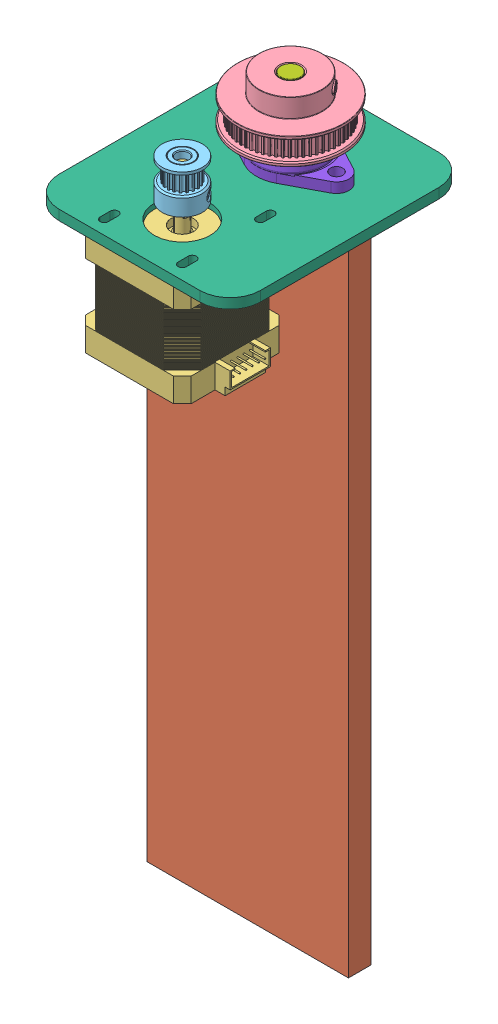
SolidWorks assembly Eje_Z, configuration Predeterminado. Lengths in mm.
Overall size (80 283.35 95).
15 component instances, 12 part files, 24 mates.
Components (placement in the parent):
- Eje_Z_guia_MGN12^Eje_Z-1: Eje_Z_guia_MGN12^Eje_Z [Predeterminado] at (56.2598 -105.1519 134.6514) x (1 0 0) z (0 1 0) size (9 6.61 250) (virtual)
- Copia de Placa_Motor^Eje_Z-1: Copia de Placa_Motor^Eje_Z [Predeterminado] at (70.7598 -105.1519 145.8457) x (-1 0 0) z (0 0 -1) size (80 250 9) (virtual)
-  Nema 17HS4401-S^Eje_Z-1:  Nema 17HS4401-S^Eje_Z [Varsayılan] at (30.7598 104.6481 171.8457) x (0 0 1) z (0 1 0) size (42 48 63.23) (virtual)
-  GT2_60T_8_6^Eje_Z-1:  GT2_60T_8_6^Eje_Z [Default] at (30.7598 170.6981 128.8457) x (0.816489 0 -0.577361) z (0 -1 0) size (42 42 18) (virtual)
- GT2_20T^Eje_Z-1: GT2_20T^Eje_Z [Конфигурация1] at (30.7598 154.7481 171.8457) x (0 1 0) z (-0.516573 0 -0.856243) size (16 16 16) (virtual)
- soporte_motor_Z-1: soporte_motor_Z [Predeterminado] at (-9.2402 148.8481 192.8457) x (0 0 -1) z (0 -1 0) size (95 80 4)
- Copia de LeadScrew 8mm x 2mmPitch_eje_Z^Eje_Z-1: Copia de LeadScrew 8mm x 2mmPitch_eje_Z^Eje_Z [Default] at (30.7598 178.1981 128.8457) x (0.80721 0 -0.590265) z (0 1 0) size (8 8 283) (virtual)
- Copia de KFL08^Eje_Z-1: Copia de KFL08^Eje_Z [Varsayılan] at (30.7598 148.8481 128.8457) size (46.5 11.35 27) (virtual)
  - Copia de FLANGE^Copia de KFL08_Eje_Z-1: Copia de FLANGE^Copia de KFL08_Eje_Z [Default] at origin size (46.5 8.5 27) (virtual)
  - Copia de BEARING^Copia de KFL08_Eje_Z-1: Copia de BEARING^Copia de KFL08_Eje_Z [Default] at (0 4 0) x (1 0 0) z (0 -1 0) size (22 22 10.85) (virtual)
  - socket set screw cone point_am-1: socket set screw cone point_am [B18.3.6M - M2.5 x 0.45 x 2 Hex Socket Cone Pt. SS --S] at (0 9.425 5.45) x (0 0 -1) z (1 0 0) size (2 2.5 2.5)
  - socket set screw cone point_am-2: socket set screw cone point_am [B18.3.6M - M2.5 x 0.45 x 2 Hex Socket Cone Pt. SS --S] at (5.45 9.425 0) x (-1 0 0) z (0 0 -1) size (2 2.5 2.5)
- Eje_Z_guia_MGN12^Eje_Z-2: Eje_Z_guia_MGN12^Eje_Z [Predeterminado] at (5.2598 -105.1519 134.6514) x (1 0 0) z (0 1 0) size (9 6.61 250) (virtual)
- NEMA 23HS7430-1: NEMA 23HS7430 [По умолчанию] at (40.5598 155.7481 54.6457) x (1 0 0) z (0 -1 0) size (58.4 56.4 95.6) (hidden)
- Pieza1^Eje_Z-1: Pieza1^Eje_Z [Predeterminado] at origin (virtual)
Mates (geometry in assembly coordinates):
- Coincidente239: coincident anti-aligned: plane of Copia de Placa_Motor^Eje_Z-1 through (70.7598 144.8481 137.8457) normal (0 1 0); plane of soporte_motor_Z-1 through (-9.2402 144.8481 192.8457) normal (0 -1 0)
- Coincidente240: coincident aligned: plane of Copia de Placa_Motor^Eje_Z-1 through (-9.2402 -105.1519 137.8457) normal (-1 0 0); plane of soporte_motor_Z-1 through (-9.2402 144.8481 192.8457) normal (-1 0 0)
- Distancia1: distance = 47 mm aligned: plane of Copia de Placa_Motor^Eje_Z-1 through (70.7598 -105.1519 145.8457) normal (0 0 1); plane of soporte_motor_Z-1 through (-9.2402 144.8481 192.8457) normal (0 0 1)
- Coincidente242: coincident anti-aligned: plane of  Nema 17HS4401-S^Eje_Z-1 through (30.7598 144.8481 171.8457) normal (0 1 0); plane of soporte_motor_Z-1 through (-9.2402 144.8481 192.8457) normal (0 -1 0)
- Coincidente245: coincident anti-aligned: plane of soporte_motor_Z-1 through (-9.2402 148.8481 192.8457) normal (0 1 0); plane of Copia de KFL08^Eje_Z-1/Copia de FLANGE^Copia de KFL08_Eje_Z-1 through (49.0098 148.8481 128.8457) normal (0 -1 0)
- Concéntrica10: concentric anti-aligned: cylinder of Copia de LeadScrew 8mm x 2mmPitch_eje_Z^Eje_Z-1 through (30.7598 -104.8019 128.8457) axis (0 1 0) radius 4; cylinder of Copia de KFL08^Eje_Z-1/Copia de BEARING^Copia de KFL08_Eje_Z-1 through (30.7598 149.3481 128.8457) axis (0 -1 0) radius 4
- Concéntrica11: concentric aligned: cylinder of  GT2_60T_8_6^Eje_Z-1 through (30.7598 140.6981 128.8457) axis (0 1 0) radius 4; cylinder of Copia de LeadScrew 8mm x 2mmPitch_eje_Z^Eje_Z-1 through (30.7598 -104.8019 128.8457) axis (0 1 0) radius 4
- Concéntrica12: concentric anti-aligned: cylinder of  Nema 17HS4401-S^Eje_Z-1 through (30.7598 167.8481 171.8457) axis (0 -1 0) radius 2.5; cylinder of GT2_20T^Eje_Z-1 through (30.7598 154.7481 171.8457) axis (0 1 0) radius 2.5
- Coincidente248: coincident aligned: plane of  GT2_60T_8_6^Eje_Z-1 through (30.7598 169.1981 128.8457) normal (0 -1 0); plane of GT2_20T^Eje_Z-1 through (30.7598 169.1981 171.8457) normal (0 -1 0)
- Coincidente249: coincident aligned: plane of  Nema 17HS4401-S^Eje_Z-1 through (13.2598 114.1481 192.8457) normal (0 0 1); plane of soporte_motor_Z-1 through (-9.2402 144.8481 192.8457) normal (0 0 1)
- Distancia2: distance = 19 mm aligned: plane of  Nema 17HS4401-S^Eje_Z-1 through (9.7598 114.1481 154.3457) normal (-1 0 0); plane of soporte_motor_Z-1 through (-9.2402 144.8481 192.8457) normal (-1 0 0)
- Coincidente250: coincident anti-aligned: plane of  GT2_60T_8_6^Eje_Z-1 through (30.7598 160.1981 128.8457) normal (0 -1 0); plane of Copia de KFL08^Eje_Z-1/Copia de BEARING^Copia de KFL08_Eje_Z-1 through (30.7598 160.1981 133.1457) normal (0 1 0)
- Concéntrica13: concentric aligned: cylinder of soporte_motor_Z-1 through (30.7598 144.8481 128.8457) axis (0 1 0) radius 6; cylinder of Copia de LeadScrew 8mm x 2mmPitch_eje_Z^Eje_Z-1 through (30.7598 -104.8019 128.8457) axis (0 1 0) radius 4
- Coincidente252: coincident aligned: plane of  GT2_60T_8_6^Eje_Z-1 through (30.7598 178.1981 128.8457) normal (0 1 0); plane of Copia de LeadScrew 8mm x 2mmPitch_eje_Z^Eje_Z-1 through (30.7598 178.1981 128.8457) normal (0 1 0)
- Concéntrica14: concentric aligned: cylinder of soporte_motor_Z-1 through (49.0098 144.8481 128.8457) axis (0 1 0) radius 1.625; cylinder of Copia de KFL08^Eje_Z-1/Copia de FLANGE^Copia de KFL08_Eje_Z-1 through (49.0098 152.8481 128.8457) axis (0 1 0) radius 2.5
- Coincidente253: coincident aligned: plane of NEMA 23HS7430-1 through (40.5598 157.3481 54.6457) normal (0 1 0); plane of Copia de KFL08^Eje_Z-1/Copia de FLANGE^Copia de KFL08_Eje_Z-1 through (18.0848 157.3481 128.8457) normal (0 1 0)
- Distancia3: distance = 2 mm aligned: plane of NEMA 23HS7430-1 through (68.7598 145.7481 26.4457) normal (1 0 0); plane of soporte_motor_Z-1 through (70.7598 144.8481 192.8457) normal (1 0 0)
- Distancia4: distance = 55 mm anti-aligned: plane of Copia de Placa_Motor^Eje_Z-1 through (70.7598 -105.1519 137.8457) normal (0 0 -1); plane of NEMA 23HS7430-1 through (12.3598 145.7481 82.8457) normal (0 0 1)
- Coincidente254: coincident anti-aligned: plane of Eje_Z_guia_MGN12^Eje_Z-1 through (56.2598 -105.1519 137.8457) normal (0 0 1); plane of Copia de Placa_Motor^Eje_Z-1 through (70.7598 -105.1519 137.8457) normal (0 0 -1)
- Coincidente255: coincident anti-aligned: plane of Eje_Z_guia_MGN12^Eje_Z-1 through (60.7598 144.8481 137.8457) normal (1 0 0); plane of Copia de Placa_Motor^Eje_Z-1 through (60.7598 -105.1519 136.8457) normal (-1 0 0)
- Coincidente256: coincident aligned: plane of Eje_Z_guia_MGN12^Eje_Z-1 through (56.2598 -105.1519 134.6514) normal (0 -1 0); plane of Copia de Placa_Motor^Eje_Z-1 through (70.7598 -105.1519 137.8457) normal (0 -1 0)
- Coincidente257: coincident aligned: plane of Copia de Placa_Motor^Eje_Z-1 through (70.7598 -105.1519 137.8457) normal (0 -1 0); plane of Eje_Z_guia_MGN12^Eje_Z-2 through (5.2598 -105.1519 134.6514) normal (0 -1 0)
- Coincidente258: coincident anti-aligned: plane of Copia de Placa_Motor^Eje_Z-1 through (0.7598 -105.1519 136.8457) normal (1 0 0); plane of Eje_Z_guia_MGN12^Eje_Z-2 through (0.7598 -355.1519 137.8457) normal (-1 0 0)
- Coincidente259: coincident anti-aligned: plane of Copia de Placa_Motor^Eje_Z-1 through (70.7598 -105.1519 137.8457) normal (0 0 -1); plane of Eje_Z_guia_MGN12^Eje_Z-2 through (5.2598 -105.1519 137.8457) normal (0 0 1)
